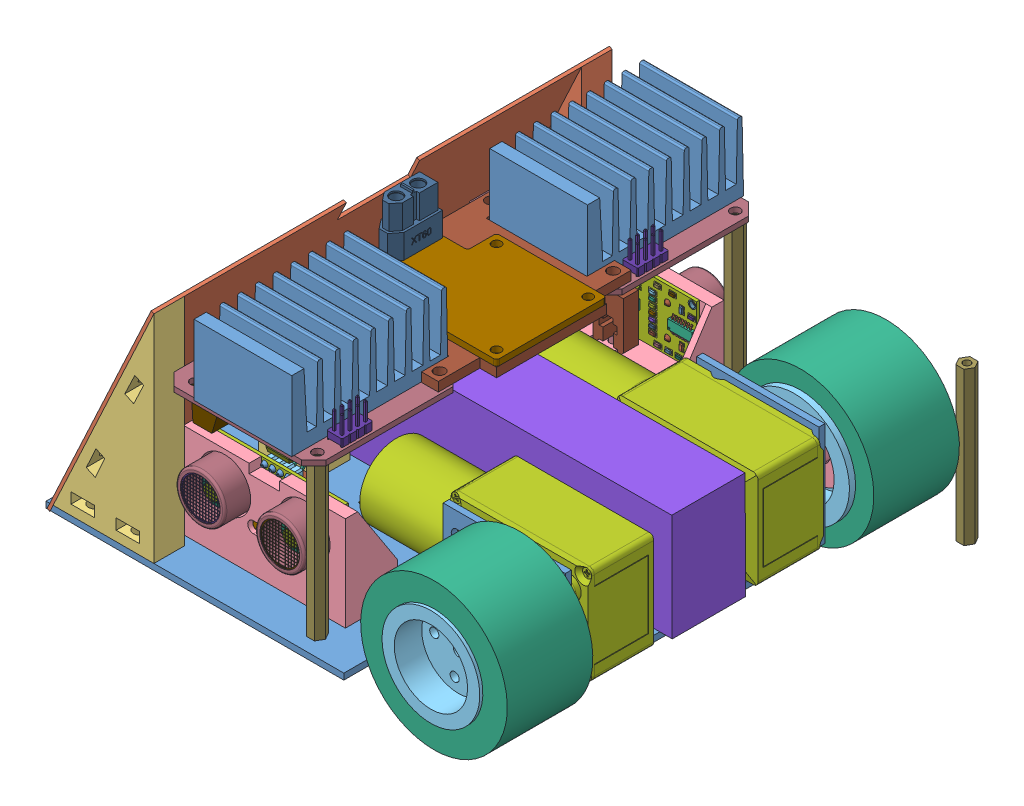
SolidWorks assembly sumover4, configuration Default. Lengths in mm.
Overall size (156.71 90.51 158.03).
240 component instances, 83 part files, 55 mates.
Components (placement in the parent):
- de_ver4-1: de_ver4 [Default] at (25.2124 85.45 125.8275) size (137.5 34 150)
- part_do_mui_phai-1: part_do_mui_phai [Default] at (-8.2076 87.45 60.8275) x (-1 0 0) z (0 0 -1) size (33 75.77 10)
- part_do_mui-1: part_do_mui [Default] at (-8.2076 87.45 200.8275) x (-1 0 0) z (0 0 -1) size (33 75.77 10)
- cum_mat_hai_ben-1: cum_mat_hai_ben [Default] at (15.9657 73.6076 21.8207) size (53 36.57 25)
  - ga lap ultrasonic v6-1: ga lap ultrasonic v6 [Default] at (-15.0838 26.1355 42.0068) size (53 31 17)
  - HC-04HC-04-1: HC-04HC-04 [Default] at (-1.0033 34.8424 47.0068) x (1 0 0) z (0 0 -1) size (45 25.57 17.46)
    - HC-04HC-04.stp-1: HC-04HC-04.stp [Default] at origin size (45 25.57 17.46)
      - HC-04Array.stp-1: HC-04Array.stp [Default] at origin size (10.16 2.54 2.54)
      - HC-04Array001.stp-1: HC-04Array001.stp [Default] at (0 0 1) size (8.32 7.52 6.46)
      - HC-04Placa.stp-1: HC-04Placa.stp [Default] at origin size (45 20 1)
      - HC-04Pad003.stp-1: HC-04Pad003.stp [Default] at (0 0 1) size (10.52 3.38 0.2)
      - HC-04Fillet.stp-1: HC-04Fillet.stp [Default] at (0 0 1) size (10.1 2.84 3)
      - HC-04Array002.stp-1: HC-04Array002.stp [Default] at origin size (9.62 2 1)
      - HC-04Array003.stp-1: HC-04Array003.stp [Default] at (0 0 1) size (28 12 0.8)
      - HC-04Fusion.stp-1: HC-04Fusion.stp [Default] at origin size (6 2 1)
      - HC-04Fillet001.stp-1: HC-04Fillet001.stp [Default] at (0 0 1) size (42 16 12)
      - HC-04Pad005.stp-1: HC-04Pad005.stp [Default] at (0 0 1) size (39.16 13 0.2)
      - HC-04Pad006.stp-1: HC-04Pad006.stp [Default] at (0 0 1) size (35.01 9.04 7)
      - HC-04Fusion001.stp-1: HC-04Fusion001.stp [Default] at (0 0 8) size (31 5 1.5)
      - HC-04Clone_of_Fusion002.stp-1: HC-04Clone_of_Fusion002.stp [Default] at (47.2 -5.5 12.6) size (13 13 0.15)
      - HC-04Clone_of_Fusion003.stp-1: HC-04Clone_of_Fusion003.stp [Default] at (21.2 -5.5 12.6) size (13 13 0.15)
      - HC-04Array005.stp-1: HC-04Array005.stp [Default] at origin size (9.62 2 1)
      - HC-04Array002002.stp-1: HC-04Array002002.stp [Default] at (-5.9 0.1 0.15) size (6.57 1.4 0.56)
      - HC-04Clone_of_Array002002.stp-1: HC-04Clone_of_Array002002.stp [Default] at (-23.9 0.1 0.15) size (6.57 1.4 0.56)
      - HC-04Array002003.stp-1: HC-04Array002003.stp [Default] at (-6.05 0 0.15) size (6.57 1.4 0.56)
      - HC-04Clone_of_Array002003.stp-1: HC-04Clone_of_Array002003.stp [Default] at (-24.05 0 0.15) size (6.57 1.4 0.56)
      - HC-04Integrados.stp-1: HC-04Integrados.stp [Default] at origin size (42.14 9 1)
      - HC-04ShapeString.stp-1: HC-04ShapeString.stp [Default] at (-3.2 -7 1.01) x (0 1 0) z (0 0 1) size (2.53 1.13 0.01)
      - HC-04ShapeString001.stp-1: HC-04ShapeString001.stp [Default] at (-0.6 -7 1.01) x (0 1 0) z (0 0 1) size (2.66 1.45 0.01)
      - HC-04ShapeString002.stp-1: HC-04ShapeString002.stp [Default] at (1.9 -7 1.01) x (0 1 0) z (0 0 1) size (3.21 1.16 0.01)
      - HC-04ShapeString003.stp-1: HC-04ShapeString003.stp [Default] at (4.5 -7 1.01) x (0 1 0) z (0 0 1) size (2.71 1.16 0.01)
      - HC-04ShapeString004.stp-1: HC-04ShapeString004.stp [Default] at (-19.5 -9.3 1.01) size (1.84 2.34 0.01)
      - HC-04ShapeString005.stp-1: HC-04ShapeString005.stp [Default] at (17.5 -9.3 1.01) size (1.82 2.34 0.01)
      - HC-04ShapeString006.stp-1: HC-04ShapeString006.stp [Default] at (-3 3.7 1.01) size (5.52 1.41 0.01)
      - HC-04Pad008.stp-1: HC-04Pad008.stp [Default] at (0 0 -0.01) size (44.56 19.6 1.02)
      - HC-04Scale004.stp-1: HC-04Scale004.stp [Default] at (-1.9 -21.5 -1.5) x (0 1 0) z (0 0 1) size (0.8 1.77 0.5)
      - HC-04Scale027.stp-1: HC-04Scale027.stp [Default] at (-1.9 -10.2323 -1.5) x (0 1 0) z (0 0 1) size (0.8 1.77 0.5)
      - HC-04Scale028.stp-1: HC-04Scale028.stp [Default] at (8.5984 -21.5 -1.5) x (0 1 0) z (0 0 1) size (0.8 1.77 0.5)
      - HC-04Scale029.stp-1: HC-04Scale029.stp [Default] at (8.5984 -19.5867 -1.5) x (0 1 0) z (0 0 1) size (0.8 1.77 0.5)
      - HC-04Scale030.stp-1: HC-04Scale030.stp [Default] at (8.5984 -17.5982 -1.5) x (0 1 0) z (0 0 1) size (0.8 1.77 0.5)
      - HC-04Scale031.stp-1: HC-04Scale031.stp [Default] at (8.5984 -15.6427 -1.5) x (0 1 0) z (0 0 1) size (0.8 1.77 0.5)
      - HC-04Scale032.stp-1: HC-04Scale032.stp [Default] at (8.5984 -11.6848 -1.5) x (0 1 0) z (0 0 1) size (0.8 1.77 0.5)
      - HC-04Scale033.stp-1: HC-04Scale033.stp [Default] at (-26.74 -2 -1.5) x (0 1 0) z (0 0 1) size (0.8 1.85 0.5)
      - HC-04Scale034.stp-1: HC-04Scale034.stp [Default] at (24.9371 -21.5 -1.5) x (0 1 0) z (0 0 1) size (0.8 1.77 0.5)
      - HC-04Scale035.stp-1: HC-04Scale035.stp [Default] at (24.9691 -19.5867 -1.5) x (0 1 0) z (0 0 1) size (0.8 1.77 0.5)
      - HC-04Scale036.stp-1: HC-04Scale036.stp [Default] at (24.9742 -17.5982 -1.5) x (0 1 0) z (0 0 1) size (0.8 1.77 0.5)
      - HC-04Scale037.stp-1: HC-04Scale037.stp [Default] at (-10.4013 -2 -1.5) x (0 1 0) z (0 0 1) size (0.8 1.85 0.5)
      - HC-04Scale038.stp-1: HC-04Scale038.stp [Default] at (-10.4013 -3.9266 -1.5) x (0 1 0) z (0 0 1) size (0.8 1.85 0.5)
      - HC-04Scale039.stp-1: HC-04Scale039.stp [Default] at (-10.4013 -0.0734 -1.5) x (0 1 0) z (0 0 1) size (0.8 1.85 0.5)
      - HC-04Scale040.stp-1: HC-04Scale040.stp [Default] at (24.9742 -9.855 -1.5) x (0 1 0) z (0 0 1) size (0.8 1.77 0.5)
      - HC-04Scale041.stp-1: HC-04Scale041.stp [Default] at (26.5673 -24.0564 -1.5) x (0 1 0) z (0 0 1) size (0.8 1.77 0.5)
      - HC-04Scale042.stp-1: HC-04Scale042.stp [Default] at (26.5673 -7.3333 -1.5) x (0 1 0) z (0 0 1) size (0.8 1.77 0.5)
      - HC-04Scale043.stp-1: HC-04Scale043.stp [Default] at (30.1435 -7.3333 -1.5) x (0 1 0) z (0 0 1) size (0.8 1.77 0.5)
      - HC-04Scale044.stp-1: HC-04Scale044.stp [Default] at (33.5459 -7.3333 -1.5) x (0 1 0) z (0 0 1) size (0.8 1.77 0.5)
      - HC-04Scale045.stp-1: HC-04Scale045.stp [Default] at (37.7181 -11.1827 -1.5) x (0 1 0) z (0 0 1) size (0.8 1.77 0.5)
      - HC-04Scale046.stp-1: HC-04Scale046.stp [Default] at (37.7181 -20.5932 -1.5) x (0 1 0) z (0 0 1) size (0.8 1.77 0.5)
      - HC-04Scale047.stp-1: HC-04Scale047.stp [Default] at (-3.9042 -12.3288 -1.5) x (0 1 0) z (0 0 1) size (0.8 1.85 0.5)
      - HC-04Scale048.stp-1: HC-04Scale048.stp [Default] at (13.5402 13.2894 -1.5) size (0.8 1.85 0.5)
      - HC-04Scale049.stp-1: HC-04Scale049.stp [Default] at (13.5402 23.7909 -1.5) size (0.8 1.85 0.5)
      - HC-04Pad009.stp-1: HC-04Pad009.stp [Default] x (1 0 0) z (0 0 -1) size (42.21 18.43 0.01)
      - HC-04ShapeString007.stp-1: HC-04ShapeString007.stp [Default] at (-3.2 -7 -0.1) x (0 1 0) z (0 0 1) size (2.53 1.13 0.01)
      - HC-04ShapeString008.stp-1: HC-04ShapeString008.stp [Default] at (-0.6 -7 -0.1) x (0 1 0) z (0 0 1) size (2.66 1.45 0.01)
      - HC-04ShapeString009.stp-1: HC-04ShapeString009.stp [Default] at (1.9 -7 -0.1) x (0 1 0) z (0 0 1) size (3.21 1.16 0.01)
      - HC-04ShapeString010.stp-1: HC-04ShapeString010.stp [Default] at (4.5 -7 -0.1) x (0 1 0) z (0 0 1) size (2.71 1.16 0.01)
      - HC-04Fusion002.stp-1: HC-04Fusion002.stp [Default] at origin size (5.7 7.57 0.56)
      - HC-04ShapeString011.stp-1: HC-04ShapeString011.stp [Default] at (-17.5 8.4 1.1) size (7.91 1.16 0.01)
      - HC-04ShapeString012.stp-1: HC-04ShapeString012.stp [Default] at (-7.5 8 -0.1) x (-1 0 0) z (0 0 -1) size (7.91 1.16 0.01)
  - 12.ganh-1: 12.ganh [Default] at (-1.0033 30.7424 48.5068) x (1 0 0) z (0 -1 0) size (10 5 19)
- cum_mat_hai_ben-2: cum_mat_hai_ben [Default] at (13.9591 73.6076 229.8343) x (-1 0 0) z (0 0 -1) size (53 36.57 25)
  - ga lap ultrasonic v6-1: ga lap ultrasonic v6 [Default] at (-15.0838 26.1355 42.0068) size (53 31 17)
  - HC-04HC-04-1: HC-04HC-04 [Default] at (-1.0033 34.8424 47.0068) x (1 0 0) z (0 0 -1) size (45 25.57 17.46)
    - HC-04HC-04.stp-1: HC-04HC-04.stp [Default] at origin size (45 25.57 17.46)
      - HC-04Array.stp-1: HC-04Array.stp [Default] at origin size (10.16 2.54 2.54)
      - HC-04Array001.stp-1: HC-04Array001.stp [Default] at (0 0 1) size (8.32 7.52 6.46)
      - HC-04Placa.stp-1: HC-04Placa.stp [Default] at origin size (45 20 1)
      - HC-04Pad003.stp-1: HC-04Pad003.stp [Default] at (0 0 1) size (10.52 3.38 0.2)
      - HC-04Fillet.stp-1: HC-04Fillet.stp [Default] at (0 0 1) size (10.1 2.84 3)
      - HC-04Array002.stp-1: HC-04Array002.stp [Default] at origin size (9.62 2 1)
      - HC-04Array003.stp-1: HC-04Array003.stp [Default] at (0 0 1) size (28 12 0.8)
      - HC-04Fusion.stp-1: HC-04Fusion.stp [Default] at origin size (6 2 1)
      - HC-04Fillet001.stp-1: HC-04Fillet001.stp [Default] at (0 0 1) size (42 16 12)
      - HC-04Pad005.stp-1: HC-04Pad005.stp [Default] at (0 0 1) size (39.16 13 0.2)
      - HC-04Pad006.stp-1: HC-04Pad006.stp [Default] at (0 0 1) size (35.01 9.04 7)
      - HC-04Fusion001.stp-1: HC-04Fusion001.stp [Default] at (0 0 8) size (31 5 1.5)
      - HC-04Clone_of_Fusion002.stp-1: HC-04Clone_of_Fusion002.stp [Default] at (47.2 -5.5 12.6) size (13 13 0.15)
      - HC-04Clone_of_Fusion003.stp-1: HC-04Clone_of_Fusion003.stp [Default] at (21.2 -5.5 12.6) size (13 13 0.15)
      - HC-04Array005.stp-1: HC-04Array005.stp [Default] at origin size (9.62 2 1)
      - HC-04Array002002.stp-1: HC-04Array002002.stp [Default] at (-5.9 0.1 0.15) size (6.57 1.4 0.56)
      - HC-04Clone_of_Array002002.stp-1: HC-04Clone_of_Array002002.stp [Default] at (-23.9 0.1 0.15) size (6.57 1.4 0.56)
      - HC-04Array002003.stp-1: HC-04Array002003.stp [Default] at (-6.05 0 0.15) size (6.57 1.4 0.56)
      - HC-04Clone_of_Array002003.stp-1: HC-04Clone_of_Array002003.stp [Default] at (-24.05 0 0.15) size (6.57 1.4 0.56)
      - HC-04Integrados.stp-1: HC-04Integrados.stp [Default] at origin size (42.14 9 1)
      - HC-04ShapeString.stp-1: HC-04ShapeString.stp [Default] at (-3.2 -7 1.01) x (0 1 0) z (0 0 1) size (2.53 1.13 0.01)
      - HC-04ShapeString001.stp-1: HC-04ShapeString001.stp [Default] at (-0.6 -7 1.01) x (0 1 0) z (0 0 1) size (2.66 1.45 0.01)
      - HC-04ShapeString002.stp-1: HC-04ShapeString002.stp [Default] at (1.9 -7 1.01) x (0 1 0) z (0 0 1) size (3.21 1.16 0.01)
      - HC-04ShapeString003.stp-1: HC-04ShapeString003.stp [Default] at (4.5 -7 1.01) x (0 1 0) z (0 0 1) size (2.71 1.16 0.01)
      - HC-04ShapeString004.stp-1: HC-04ShapeString004.stp [Default] at (-19.5 -9.3 1.01) size (1.84 2.34 0.01)
      - HC-04ShapeString005.stp-1: HC-04ShapeString005.stp [Default] at (17.5 -9.3 1.01) size (1.82 2.34 0.01)
      - HC-04ShapeString006.stp-1: HC-04ShapeString006.stp [Default] at (-3 3.7 1.01) size (5.52 1.41 0.01)
      - HC-04Pad008.stp-1: HC-04Pad008.stp [Default] at (0 0 -0.01) size (44.56 19.6 1.02)
      - HC-04Scale004.stp-1: HC-04Scale004.stp [Default] at (-1.9 -21.5 -1.5) x (0 1 0) z (0 0 1) size (0.8 1.77 0.5)
      - HC-04Scale027.stp-1: HC-04Scale027.stp [Default] at (-1.9 -10.2323 -1.5) x (0 1 0) z (0 0 1) size (0.8 1.77 0.5)
      - HC-04Scale028.stp-1: HC-04Scale028.stp [Default] at (8.5984 -21.5 -1.5) x (0 1 0) z (0 0 1) size (0.8 1.77 0.5)
      - HC-04Scale029.stp-1: HC-04Scale029.stp [Default] at (8.5984 -19.5867 -1.5) x (0 1 0) z (0 0 1) size (0.8 1.77 0.5)
      - HC-04Scale030.stp-1: HC-04Scale030.stp [Default] at (8.5984 -17.5982 -1.5) x (0 1 0) z (0 0 1) size (0.8 1.77 0.5)
      - HC-04Scale031.stp-1: HC-04Scale031.stp [Default] at (8.5984 -15.6427 -1.5) x (0 1 0) z (0 0 1) size (0.8 1.77 0.5)
      - HC-04Scale032.stp-1: HC-04Scale032.stp [Default] at (8.5984 -11.6848 -1.5) x (0 1 0) z (0 0 1) size (0.8 1.77 0.5)
      - HC-04Scale033.stp-1: HC-04Scale033.stp [Default] at (-26.74 -2 -1.5) x (0 1 0) z (0 0 1) size (0.8 1.85 0.5)
      - HC-04Scale034.stp-1: HC-04Scale034.stp [Default] at (24.9371 -21.5 -1.5) x (0 1 0) z (0 0 1) size (0.8 1.77 0.5)
      - HC-04Scale035.stp-1: HC-04Scale035.stp [Default] at (24.9691 -19.5867 -1.5) x (0 1 0) z (0 0 1) size (0.8 1.77 0.5)
      - HC-04Scale036.stp-1: HC-04Scale036.stp [Default] at (24.9742 -17.5982 -1.5) x (0 1 0) z (0 0 1) size (0.8 1.77 0.5)
      - HC-04Scale037.stp-1: HC-04Scale037.stp [Default] at (-10.4013 -2 -1.5) x (0 1 0) z (0 0 1) size (0.8 1.85 0.5)
      - HC-04Scale038.stp-1: HC-04Scale038.stp [Default] at (-10.4013 -3.9266 -1.5) x (0 1 0) z (0 0 1) size (0.8 1.85 0.5)
      - HC-04Scale039.stp-1: HC-04Scale039.stp [Default] at (-10.4013 -0.0734 -1.5) x (0 1 0) z (0 0 1) size (0.8 1.85 0.5)
      - HC-04Scale040.stp-1: HC-04Scale040.stp [Default] at (24.9742 -9.855 -1.5) x (0 1 0) z (0 0 1) size (0.8 1.77 0.5)
      - HC-04Scale041.stp-1: HC-04Scale041.stp [Default] at (26.5673 -24.0564 -1.5) x (0 1 0) z (0 0 1) size (0.8 1.77 0.5)
      - HC-04Scale042.stp-1: HC-04Scale042.stp [Default] at (26.5673 -7.3333 -1.5) x (0 1 0) z (0 0 1) size (0.8 1.77 0.5)
      - HC-04Scale043.stp-1: HC-04Scale043.stp [Default] at (30.1435 -7.3333 -1.5) x (0 1 0) z (0 0 1) size (0.8 1.77 0.5)
      - HC-04Scale044.stp-1: HC-04Scale044.stp [Default] at (33.5459 -7.3333 -1.5) x (0 1 0) z (0 0 1) size (0.8 1.77 0.5)
      - HC-04Scale045.stp-1: HC-04Scale045.stp [Default] at (37.7181 -11.1827 -1.5) x (0 1 0) z (0 0 1) size (0.8 1.77 0.5)
      - HC-04Scale046.stp-1: HC-04Scale046.stp [Default] at (37.7181 -20.5932 -1.5) x (0 1 0) z (0 0 1) size (0.8 1.77 0.5)
      - HC-04Scale047.stp-1: HC-04Scale047.stp [Default] at (-3.9042 -12.3288 -1.5) x (0 1 0) z (0 0 1) size (0.8 1.85 0.5)
      - HC-04Scale048.stp-1: HC-04Scale048.stp [Default] at (13.5402 13.2894 -1.5) size (0.8 1.85 0.5)
      - HC-04Scale049.stp-1: HC-04Scale049.stp [Default] at (13.5402 23.7909 -1.5) size (0.8 1.85 0.5)
      - HC-04Pad009.stp-1: HC-04Pad009.stp [Default] x (1 0 0) z (0 0 -1) size (42.21 18.43 0.01)
      - HC-04ShapeString007.stp-1: HC-04ShapeString007.stp [Default] at (-3.2 -7 -0.1) x (0 1 0) z (0 0 1) size (2.53 1.13 0.01)
      - HC-04ShapeString008.stp-1: HC-04ShapeString008.stp [Default] at (-0.6 -7 -0.1) x (0 1 0) z (0 0 1) size (2.66 1.45 0.01)
      - HC-04ShapeString009.stp-1: HC-04ShapeString009.stp [Default] at (1.9 -7 -0.1) x (0 1 0) z (0 0 1) size (3.21 1.16 0.01)
      - HC-04ShapeString010.stp-1: HC-04ShapeString010.stp [Default] at (4.5 -7 -0.1) x (0 1 0) z (0 0 1) size (2.71 1.16 0.01)
      - HC-04Fusion002.stp-1: HC-04Fusion002.stp [Default] at origin size (5.7 7.57 0.56)
      - HC-04ShapeString011.stp-1: HC-04ShapeString011.stp [Default] at (-17.5 8.4 1.1) size (7.91 1.16 0.01)
      - HC-04ShapeString012.stp-1: HC-04ShapeString012.stp [Default] at (-7.5 8 -0.1) x (-1 0 0) z (0 0 -1) size (7.91 1.16 0.01)
  - 12.ganh-1: 12.ganh [Default] at (-1.0033 30.7424 48.5068) x (1 0 0) z (0 -1 0) size (10 5 19)
- truc_dong_50mm-1: truc_dong_50mm [Default] at (38.7124 87.45 194.2275) size (5.31 50 4.6)
- truc_dong_50mm-2: truc_dong_50mm [Default] at (-1.2876 87.45 154.2275) x (-0.99996 0 -0.00896) z (0.00896 0 -0.99996) size (5.31 50 4.6)
- truc_dong_50mm-3: truc_dong_50mm [Default] at (-1.2876 87.45 97.4275) x (-0.99996 0 -0.00896) z (0.00896 0 -0.99996) size (5.31 50 4.6)
- truc_dong_50mm-4: truc_dong_50mm [Default] at (38.7124 87.45 57.4275) x (-0.99996 0 -0.00896) z (0.00896 0 -0.99996) size (5.31 50 4.6)
- BTS_co_tan_nhiet-1: BTS_co_tan_nhiet [Default] at (-58.0066 153.9561 222.7544) x (0 0 1) z (1 0 0) size (51 42.4 49.96)
  - 8.BTS7960 43A HIGH POWER H BRIDGE MODULE-1: 8.BTS7960 43A HIGH POWER H BRIDGE MODULE [Default] at (-48.5269 14.8061 75.419) size (49.5 27.9 49.96)
    - PCB, BTS7960 43A HIGH POWER H BRIDGE MODULE-1: PCB, BTS7960 43A HIGH POWER H BRIDGE MODULE [Default] at origin size (49.5 1.7 49.8)
    - ALUMINUM ELECTROLYTIC CAPACITOR, 330 uF, BTS7960 43A HIGH POWER H BRIDGE MODULE-1: ALUMINUM ELECTROLYTIC CAPACITOR, 330 uF, BTS7960 43A HIGH POWER H BRIDGE MODULE [Default] at (-10.75 1.8 -19.85) x (0.999469 0 -0.032584) z (0.032584 0 0.999469) size (10.1 18.7 10.1)
    - BTN7960 IC, BTS7960 43A HIGH POWER H BRIDGE MODULE-1: BTN7960 IC, BTS7960 43A HIGH POWER H BRIDGE MODULE [Default] at (5.95 1.7 1.8) x (-1 0 0) z (0 0 -1) size (9.6 4.6 14.9)
    - BTN7960 IC, BTS7960 43A HIGH POWER H BRIDGE MODULE-2: BTN7960 IC, BTS7960 43A HIGH POWER H BRIDGE MODULE [Default] at (-5.95 1.7 1.8) x (-1 0 0) z (0 0 -1) size (9.6 4.6 14.9)
    - NXP 74HC244D, BUFFER AND LINE DRIVER, BTS7960 43A HIGH POWER H BRIDGE MODULE-1: NXP 74HC244D, BUFFER AND LINE DRIVER, BTS7960 43A HIGH POWER H BRIDGE MODULE [Default] at (17.35 3 12.1) size (13 2.6 10.4)
    - y 8 PIN HEADER, IC, BTS7960 43A HIGH POWER H BRIDGE MODULE-1: y 8 PIN HEADER, IC, BTS7960 43A HIGH POWER H BRIDGE MODULE [Default] at (-34.78 -2.5 22.83) x (0 0 1) z (-1 0 0) size (5.08 11.6 10.16)
    - EUROSTYLE TERMINAL BLOCK 2 POS 5.0 MM RA PLUG, BTS7960 43A HIGH POWER H BRIDGE MODULE-1: EUROSTYLE TERMINAL BLOCK 2 POS 5.0 MM RA PLUG, BTS7960 43A HIGH POWER H BRIDGE MODULE [Default] at (0.75 4.2 -6.5) size (10 14.5 10.5)
    - EUROSTYLE TERMINAL BLOCK 2 POS 5.0 MM RA PLUG, BTS7960 43A HIGH POWER H BRIDGE MODULE-2: EUROSTYLE TERMINAL BLOCK 2 POS 5.0 MM RA PLUG, BTS7960 43A HIGH POWER H BRIDGE MODULE [Default] at (10.75 4.2 -6.5) size (10 14.5 10.5)
  - HEATSINK, BTS7960 43A HIGH POWER H BRIDGE MODULE-1: HEATSINK, BTS7960 43A HIGH POWER H BRIDGE MODULE [Default] at (-48.5269 14.8061 77.819) size (51 23 32.02)
- BTS_co_tan_nhiet-2: BTS_co_tan_nhiet [Default] at (-58.0066 153.9561 125.9544) x (0 0 1) z (1 0 0) size (51 42.4 49.96)
  - 8.BTS7960 43A HIGH POWER H BRIDGE MODULE-1: 8.BTS7960 43A HIGH POWER H BRIDGE MODULE [Default] at (-48.5269 14.8061 75.419) size (49.5 27.9 49.96)
    - PCB, BTS7960 43A HIGH POWER H BRIDGE MODULE-1: PCB, BTS7960 43A HIGH POWER H BRIDGE MODULE [Default] at origin size (49.5 1.7 49.8)
    - ALUMINUM ELECTROLYTIC CAPACITOR, 330 uF, BTS7960 43A HIGH POWER H BRIDGE MODULE-1: ALUMINUM ELECTROLYTIC CAPACITOR, 330 uF, BTS7960 43A HIGH POWER H BRIDGE MODULE [Default] at (-10.75 1.8 -19.85) x (0.999469 0 -0.032584) z (0.032584 0 0.999469) size (10.1 18.7 10.1)
    - BTN7960 IC, BTS7960 43A HIGH POWER H BRIDGE MODULE-1: BTN7960 IC, BTS7960 43A HIGH POWER H BRIDGE MODULE [Default] at (5.95 1.7 1.8) x (-1 0 0) z (0 0 -1) size (9.6 4.6 14.9)
    - BTN7960 IC, BTS7960 43A HIGH POWER H BRIDGE MODULE-2: BTN7960 IC, BTS7960 43A HIGH POWER H BRIDGE MODULE [Default] at (-5.95 1.7 1.8) x (-1 0 0) z (0 0 -1) size (9.6 4.6 14.9)
    - NXP 74HC244D, BUFFER AND LINE DRIVER, BTS7960 43A HIGH POWER H BRIDGE MODULE-1: NXP 74HC244D, BUFFER AND LINE DRIVER, BTS7960 43A HIGH POWER H BRIDGE MODULE [Default] at (17.35 3 12.1) size (13 2.6 10.4)
    - y 8 PIN HEADER, IC, BTS7960 43A HIGH POWER H BRIDGE MODULE-1: y 8 PIN HEADER, IC, BTS7960 43A HIGH POWER H BRIDGE MODULE [Default] at (-34.78 -2.5 22.83) x (0 0 1) z (-1 0 0) size (5.08 11.6 10.16)
    - EUROSTYLE TERMINAL BLOCK 2 POS 5.0 MM RA PLUG, BTS7960 43A HIGH POWER H BRIDGE MODULE-1: EUROSTYLE TERMINAL BLOCK 2 POS 5.0 MM RA PLUG, BTS7960 43A HIGH POWER H BRIDGE MODULE [Default] at (0.75 4.2 -6.5) size (10 14.5 10.5)
    - EUROSTYLE TERMINAL BLOCK 2 POS 5.0 MM RA PLUG, BTS7960 43A HIGH POWER H BRIDGE MODULE-2: EUROSTYLE TERMINAL BLOCK 2 POS 5.0 MM RA PLUG, BTS7960 43A HIGH POWER H BRIDGE MODULE [Default] at (10.75 4.2 -6.5) size (10 14.5 10.5)
  - HEATSINK, BTS7960 43A HIGH POWER H BRIDGE MODULE-1: HEATSINK, BTS7960 43A HIGH POWER H BRIDGE MODULE [Default] at (-48.5269 14.8061 77.819) size (51 23 32.02)
- part_chan-1: part_chan [Default] at (-26.7813 120.7534 125.8275) x (0 0 -1) z (0.906308 -0.422618 0) size (150 80.6 1)
- ga lap ultrasonic v5-1: ga lap ultrasonic v5 [Default] at (-22.5376 103.7431 139.908) x (0 0 -1) z (1 0 0) size (53 35 17)
- HC-04HC-04-1: HC-04HC-04 [Default] at (-17.5376 112.45 125.8275) x (0 0 -1) z (-1 0 0) size (45 25.57 17.46)
  - HC-04HC-04.stp-1: HC-04HC-04.stp [Default] at origin size (45 25.57 17.46)
    - HC-04Array.stp-1: HC-04Array.stp [Default] at origin size (10.16 2.54 2.54)
    - HC-04Array001.stp-1: HC-04Array001.stp [Default] at (0 0 1) size (8.32 7.52 6.46)
    - HC-04Placa.stp-1: HC-04Placa.stp [Default] at origin size (45 20 1)
    - HC-04Pad003.stp-1: HC-04Pad003.stp [Default] at (0 0 1) size (10.52 3.38 0.2)
    - HC-04Fillet.stp-1: HC-04Fillet.stp [Default] at (0 0 1) size (10.1 2.84 3)
    - HC-04Array002.stp-1: HC-04Array002.stp [Default] at origin size (9.62 2 1)
    - HC-04Array003.stp-1: HC-04Array003.stp [Default] at (0 0 1) size (28 12 0.8)
    - HC-04Fusion.stp-1: HC-04Fusion.stp [Default] at origin size (6 2 1)
    - HC-04Fillet001.stp-1: HC-04Fillet001.stp [Default] at (0 0 1) size (42 16 12)
    - HC-04Pad005.stp-1: HC-04Pad005.stp [Default] at (0 0 1) size (39.16 13 0.2)
    - HC-04Pad006.stp-1: HC-04Pad006.stp [Default] at (0 0 1) size (35.01 9.04 7)
    - HC-04Fusion001.stp-1: HC-04Fusion001.stp [Default] at (0 0 8) size (31 5 1.5)
    - HC-04Clone_of_Fusion002.stp-1: HC-04Clone_of_Fusion002.stp [Default] at (47.2 -5.5 12.6) size (13 13 0.15)
    - HC-04Clone_of_Fusion003.stp-1: HC-04Clone_of_Fusion003.stp [Default] at (21.2 -5.5 12.6) size (13 13 0.15)
    - HC-04Array005.stp-1: HC-04Array005.stp [Default] at origin size (9.62 2 1)
    - HC-04Array002002.stp-1: HC-04Array002002.stp [Default] at (-5.9 0.1 0.15) size (6.57 1.4 0.56)
    - HC-04Clone_of_Array002002.stp-1: HC-04Clone_of_Array002002.stp [Default] at (-23.9 0.1 0.15) size (6.57 1.4 0.56)
    - HC-04Array002003.stp-1: HC-04Array002003.stp [Default] at (-6.05 0 0.15) size (6.57 1.4 0.56)
    - HC-04Clone_of_Array002003.stp-1: HC-04Clone_of_Array002003.stp [Default] at (-24.05 0 0.15) size (6.57 1.4 0.56)
    - HC-04Integrados.stp-1: HC-04Integrados.stp [Default] at origin size (42.14 9 1)
    - HC-04ShapeString.stp-1: HC-04ShapeString.stp [Default] at (-3.2 -7 1.01) x (0 1 0) z (0 0 1) size (2.53 1.13 0.01)
    - HC-04ShapeString001.stp-1: HC-04ShapeString001.stp [Default] at (-0.6 -7 1.01) x (0 1 0) z (0 0 1) size (2.66 1.45 0.01)
    - HC-04ShapeString002.stp-1: HC-04ShapeString002.stp [Default] at (1.9 -7 1.01) x (0 1 0) z (0 0 1) size (3.21 1.16 0.01)
    - HC-04ShapeString003.stp-1: HC-04ShapeString003.stp [Default] at (4.5 -7 1.01) x (0 1 0) z (0 0 1) size (2.71 1.16 0.01)
    - HC-04ShapeString004.stp-1: HC-04ShapeString004.stp [Default] at (-19.5 -9.3 1.01) size (1.84 2.34 0.01)
    - HC-04ShapeString005.stp-1: HC-04ShapeString005.stp [Default] at (17.5 -9.3 1.01) size (1.82 2.34 0.01)
    - HC-04ShapeString006.stp-1: HC-04ShapeString006.stp [Default] at (-3 3.7 1.01) size (5.52 1.41 0.01)
    - HC-04Pad008.stp-1: HC-04Pad008.stp [Default] at (0 0 -0.01) size (44.56 19.6 1.02)
    - HC-04Scale004.stp-1: HC-04Scale004.stp [Default] at (-1.9 -21.5 -1.5) x (0 1 0) z (0 0 1) size (0.8 1.77 0.5)
    - HC-04Scale027.stp-1: HC-04Scale027.stp [Default] at (-1.9 -10.2323 -1.5) x (0 1 0) z (0 0 1) size (0.8 1.77 0.5)
    - HC-04Scale028.stp-1: HC-04Scale028.stp [Default] at (8.5984 -21.5 -1.5) x (0 1 0) z (0 0 1) size (0.8 1.77 0.5)
    - HC-04Scale029.stp-1: HC-04Scale029.stp [Default] at (8.5984 -19.5867 -1.5) x (0 1 0) z (0 0 1) size (0.8 1.77 0.5)
    - HC-04Scale030.stp-1: HC-04Scale030.stp [Default] at (8.5984 -17.5982 -1.5) x (0 1 0) z (0 0 1) size (0.8 1.77 0.5)
    - HC-04Scale031.stp-1: HC-04Scale031.stp [Default] at (8.5984 -15.6427 -1.5) x (0 1 0) z (0 0 1) size (0.8 1.77 0.5)
    - HC-04Scale032.stp-1: HC-04Scale032.stp [Default] at (8.5984 -11.6848 -1.5) x (0 1 0) z (0 0 1) size (0.8 1.77 0.5)
    - HC-04Scale033.stp-1: HC-04Scale033.stp [Default] at (-26.74 -2 -1.5) x (0 1 0) z (0 0 1) size (0.8 1.85 0.5)
    - HC-04Scale034.stp-1: HC-04Scale034.stp [Default] at (24.9371 -21.5 -1.5) x (0 1 0) z (0 0 1) size (0.8 1.77 0.5)
    - HC-04Scale035.stp-1: HC-04Scale035.stp [Default] at (24.9691 -19.5867 -1.5) x (0 1 0) z (0 0 1) size (0.8 1.77 0.5)
    - HC-04Scale036.stp-1: HC-04Scale036.stp [Default] at (24.9742 -17.5982 -1.5) x (0 1 0) z (0 0 1) size (0.8 1.77 0.5)
    - HC-04Scale037.stp-1: HC-04Scale037.stp [Default] at (-10.4013 -2 -1.5) x (0 1 0) z (0 0 1) size (0.8 1.85 0.5)
    - HC-04Scale038.stp-1: HC-04Scale038.stp [Default] at (-10.4013 -3.9266 -1.5) x (0 1 0) z (0 0 1) size (0.8 1.85 0.5)
    - HC-04Scale039.stp-1: HC-04Scale039.stp [Default] at (-10.4013 -0.0734 -1.5) x (0 1 0) z (0 0 1) size (0.8 1.85 0.5)
    - HC-04Scale040.stp-1: HC-04Scale040.stp [Default] at (24.9742 -9.855 -1.5) x (0 1 0) z (0 0 1) size (0.8 1.77 0.5)
    - HC-04Scale041.stp-1: HC-04Scale041.stp [Default] at (26.5673 -24.0564 -1.5) x (0 1 0) z (0 0 1) size (0.8 1.77 0.5)
    - HC-04Scale042.stp-1: HC-04Scale042.stp [Default] at (26.5673 -7.3333 -1.5) x (0 1 0) z (0 0 1) size (0.8 1.77 0.5)
    - HC-04Scale043.stp-1: HC-04Scale043.stp [Default] at (30.1435 -7.3333 -1.5) x (0 1 0) z (0 0 1) size (0.8 1.77 0.5)
    - HC-04Scale044.stp-1: HC-04Scale044.stp [Default] at (33.5459 -7.3333 -1.5) x (0 1 0) z (0 0 1) size (0.8 1.77 0.5)
    - HC-04Scale045.stp-1: HC-04Scale045.stp [Default] at (37.7181 -11.1827 -1.5) x (0 1 0) z (0 0 1) size (0.8 1.77 0.5)
    - HC-04Scale046.stp-1: HC-04Scale046.stp [Default] at (37.7181 -20.5932 -1.5) x (0 1 0) z (0 0 1) size (0.8 1.77 0.5)
    - HC-04Scale047.stp-1: HC-04Scale047.stp [Default] at (-3.9042 -12.3288 -1.5) x (0 1 0) z (0 0 1) size (0.8 1.85 0.5)
    - HC-04Scale048.stp-1: HC-04Scale048.stp [Default] at (13.5402 13.2894 -1.5) size (0.8 1.85 0.5)
    - HC-04Scale049.stp-1: HC-04Scale049.stp [Default] at (13.5402 23.7909 -1.5) size (0.8 1.85 0.5)
    - HC-04Pad009.stp-1: HC-04Pad009.stp [Default] x (1 0 0) z (0 0 -1) size (42.21 18.43 0.01)
    - HC-04ShapeString007.stp-1: HC-04ShapeString007.stp [Default] at (-3.2 -7 -0.1) x (0 1 0) z (0 0 1) size (2.53 1.13 0.01)
    - HC-04ShapeString008.stp-1: HC-04ShapeString008.stp [Default] at (-0.6 -7 -0.1) x (0 1 0) z (0 0 1) size (2.66 1.45 0.01)
    - HC-04ShapeString009.stp-1: HC-04ShapeString009.stp [Default] at (1.9 -7 -0.1) x (0 1 0) z (0 0 1) size (3.21 1.16 0.01)
    - HC-04ShapeString010.stp-1: HC-04ShapeString010.stp [Default] at (4.5 -7 -0.1) x (0 1 0) z (0 0 1) size (2.71 1.16 0.01)
    - HC-04Fusion002.stp-1: HC-04Fusion002.stp [Default] at origin size (5.7 7.57 0.56)
    - HC-04ShapeString011.stp-1: HC-04ShapeString011.stp [Default] at (-17.5 8.4 1.1) size (7.91 1.16 0.01)
    - HC-04ShapeString012.stp-1: HC-04ShapeString012.stp [Default] at (-7.5 8 -0.1) x (-1 0 0) z (0 0 -1) size (7.91 1.16 0.01)
- 12.ganh-1: 12.ganh [Default] at (-11.0376 108.35 125.8275) x (0 0 1) z (0 -1 0) size (10 5 19)
- banhxe-1: banhxe [Default] at (52.3102 164.6143 71.5756) x (0.338518 0.94096 0) z (0.94096 -0.338518 0) size (48 34 48)
  - mat_bich_phi6-1: mat_bich_phi6 [Default] at (-47.3462 1.2519 49.0772) size (22 12 22)
  - 13.LoiBanhVer3-1: 13.LoiBanhVer3 [Default] at (-47.3462 -5.7481 49.0772) x (0 -1 0) z (0 0 1) size (31 36 36)
  - 2.lop_banh_xe-1: 2.lop_banh_xe [Default] at (-47.3462 -19.7481 49.0772) x (1 0 0) z (0 1 0) size (48 48 28)
- 4.JGY370_Reduction DC Motor-6mm-2: 4.JGY370_Reduction DC Motor-6mm [Default] at (82.4624 103.45 162.3275) x (-1 0 0) z (0 1 0) size (80.2 40.2 32)
- banhxe-3: banhxe [Default] at (121.8297 47.7682 180.0794) x (0.988465 -0.151451 0) z (0.151451 0.988465 0) size (48 34 48)
  - mat_bich_phi6-1: mat_bich_phi6 [Default] at (-47.3462 1.2519 49.0772) size (22 12 22)
  - 13.LoiBanhVer3-1: 13.LoiBanhVer3 [Default] at (-47.3462 -5.7481 49.0772) x (0 -1 0) z (0 0 1) size (31 36 36)
  - 2.lop_banh_xe-1: 2.lop_banh_xe [Default] at (-47.3462 -19.7481 49.0772) x (1 0 0) z (0 1 0) size (48 48 28)
- 4.JGY370_Reduction DC Motor-6mm-3: 4.JGY370_Reduction DC Motor-6mm [Default] at (82.4624 103.45 89.3275) x (-1 0 0) z (0 -1 0) size (80.2 40.2 32)
- 9.pin-1: 9.pin [Default] at (98.3893 105.3868 125.8275) x (0.004123 -0.999992 0) z (-0.999992 -0.004123 0) size (35 24 106)
- Machchianguon-1: Machchianguon [Default] at (35.7033 112.7735 164.9544) x (-1 0 0) z (0 0 -1) size (51 21.15 36)
  - mach_chia_nguon-1: mach_chia_nguon [Default] at (-11.2591 29.3765 57.1219) size (51 2 36)
  - Component1.step-1: Component1.step [Default] at (39.7409 31.3765 46.9219) x (0 0 -1) z (0 1 0) size (15.6 7.5 21.15)
- part_do_mach_chia_nguon-1: part_do_mach_chia_nguon [Default] at (18.7124 139.15 125.8325) x (-1 0 0) z (0 1 0) size (51 63.15 3)
- truc_dong_50mm-5: truc_dong_50mm [Default] at (102.1964 71.6421 45.0966) size (5.31 50 4.6)
Mates (geometry in assembly coordinates):
- Coincident1: coincident anti-aligned: plane of de_ver4-1 through (25.2124 87.45 125.8275) normal (0 1 0); plane of part_do_mui_phai-1 through (-8.2076 87.45 50.8275) normal (0 -1 0)
- Width1: width anti-aligned: plane of part_do_mui_phai-1 through (-21.7076 82.45 53.8275) normal (0 0 -1); plane of de_ver4-1 through (-21.7076 82.45 57.8275) normal (0 0 1); plane of part_do_mui_phai-1 through (-21.7076 87.45 53.8275) normal (0 0 1); plane of de_ver4-1 through (-27.7076 87.45 57.8275) normal (0 0 -1)
- Width2: width anti-aligned: plane of part_do_mui_phai-1 through (-21.7076 82.45 53.8275) normal (1 0 0); plane of de_ver4-1 through (-27.7076 82.45 53.8275) normal (-1 0 0); plane of part_do_mui_phai-1 through (-21.7076 87.45 57.8275) normal (-1 0 0); plane of de_ver4-1 through (-27.7076 87.45 53.8275) normal (1 0 0)
- Coincident2: coincident anti-aligned: plane of de_ver4-1 through (25.2124 87.45 125.8275) normal (0 1 0); plane of part_do_mui-1 through (-8.2076 87.45 190.8275) normal (0 -1 0)
- Width3: width aligned: plane of part_do_mui-1 through (-21.7076 82.45 197.8275) normal (0 0 1); plane of de_ver4-1 through (-21.7076 82.45 193.8275) normal (0 0 -1); plane of part_do_mui-1 through (-27.7076 87.45 193.8275) normal (0 0 1); plane of de_ver4-1 through (-21.7076 87.45 197.8275) normal (0 0 -1)
- Width4: width anti-aligned: plane of de_ver4-1 through (-27.7076 87.45 197.8275) normal (1 0 0); plane of part_do_mui-1 through (-21.7076 87.45 193.8275) normal (-1 0 0); plane of de_ver4-1 through (-27.7076 82.45 193.8275) normal (-1 0 0); plane of part_do_mui-1 through (-21.7076 82.45 193.8275) normal (1 0 0)
- Coincident3: coincident anti-aligned: plane of de_ver4-1 through (25.2124 87.45 125.8275) normal (0 1 0); plane of cum_mat_hai_ben-1/ga lap ultrasonic v6-1 through (0.8819 87.45 63.8275) normal (0 -1 0)
- Concentric1: concentric anti-aligned: cylinder of de_ver4-1 through (-4.5376 87.45 75.8275) axis (0 -1 0) radius 1.75; cylinder of cum_mat_hai_ben-1/ga lap ultrasonic v6-1 through (-4.5376 93.45 75.8275) axis (0 1 0) radius 1.75
- Concentric2: concentric anti-aligned: cylinder of de_ver4-1 through (34.4624 87.45 75.8275) axis (0 -1 0) radius 1.75; cylinder of cum_mat_hai_ben-1/ga lap ultrasonic v6-1 through (34.4624 93.45 75.8275) axis (0 1 0) radius 1.75
- Coincident4: coincident anti-aligned: plane of de_ver4-1 through (25.2124 87.45 125.8275) normal (0 1 0); plane of cum_mat_hai_ben-2/ga lap ultrasonic v6-1 through (29.0429 87.45 187.8275) normal (0 -1 0)
- Concentric3: concentric anti-aligned: cylinder of de_ver4-1 through (34.4624 87.45 175.8275) axis (0 -1 0) radius 1.75; cylinder of cum_mat_hai_ben-2/ga lap ultrasonic v6-1 through (34.4624 93.45 175.8275) axis (0 1 0) radius 1.75
- Concentric4: concentric anti-aligned: cylinder of de_ver4-1 through (-4.5376 87.45 175.8275) axis (0 -1 0) radius 1.75; cylinder of cum_mat_hai_ben-2/ga lap ultrasonic v6-1 through (-4.5376 93.45 175.8275) axis (0 1 0) radius 1.75
- Coincident5: coincident anti-aligned: plane of de_ver4-1 through (25.2124 87.45 125.8275) normal (0 1 0); plane of truc_dong_50mm-1 through (38.7124 87.45 194.2275) normal (0 -1 0)
- Concentric5: concentric aligned: cylinder of de_ver4-1 through (38.7124 87.45 194.2275) axis (0 -1 0) radius 1.75; cylinder of truc_dong_50mm-1 through (38.7124 137.45 194.2275) axis (0 -1 0) radius 1.2
- Concentric6: concentric aligned: cylinder of de_ver4-1 through (-1.2876 87.45 154.2275) axis (0 -1 0) radius 1.75; cylinder of truc_dong_50mm-2 through (-1.2876 137.45 154.2275) axis (0 -1 0) radius 1.2
- Coincident6: coincident anti-aligned: plane of de_ver4-1 through (25.2124 87.45 125.8275) normal (0 1 0); plane of truc_dong_50mm-2 through (-1.2876 87.45 154.2275) normal (0 -1 0)
- Coincident7: coincident anti-aligned: plane of de_ver4-1 through (25.2124 87.45 125.8275) normal (0 1 0); plane of truc_dong_50mm-3 through (-1.2876 87.45 97.4275) normal (0 -1 0)
- Coincident8: coincident anti-aligned: plane of de_ver4-1 through (25.2124 87.45 125.8275) normal (0 1 0); plane of truc_dong_50mm-4 through (38.7124 87.45 57.4275) normal (0 -1 0)
- Concentric7: concentric aligned: cylinder of de_ver4-1 through (38.7124 87.45 57.4275) axis (0 -1 0) radius 1.75; cylinder of truc_dong_50mm-4 through (38.7124 137.45 57.4275) axis (0 -1 0) radius 1.2
- Coincident9: coincident anti-aligned: plane of truc_dong_50mm-1 through (38.7124 137.45 194.2275) normal (0 1 0); plane of BTS_co_tan_nhiet-1/8.BTS7960 43A HIGH POWER H BRIDGE MODULE-1/PCB, BTS7960 43A HIGH POWER H BRIDGE MODULE-1 through (17.4124 137.45 174.2275) normal (0 -1 0)
- Concentric9: concentric anti-aligned: circle of truc_dong_50mm-1; circle of BTS_co_tan_nhiet-1/8.BTS7960 43A HIGH POWER H BRIDGE MODULE-1/PCB, BTS7960 43A HIGH POWER H BRIDGE MODULE-1
- Concentric10: concentric aligned: cylinder of truc_dong_50mm-2 through (-1.2876 137.45 154.2275) axis (0 -1 0) radius 1.2; cylinder of BTS_co_tan_nhiet-1/8.BTS7960 43A HIGH POWER H BRIDGE MODULE-1/PCB, BTS7960 43A HIGH POWER H BRIDGE MODULE-1 through (-1.2876 137.45 154.2275) axis (0 -1 0) radius 1.6
- Coincident10: coincident anti-aligned: plane of truc_dong_50mm-3 through (-1.2876 137.45 97.4275) normal (0 1 0); plane of BTS_co_tan_nhiet-2/8.BTS7960 43A HIGH POWER H BRIDGE MODULE-1/PCB, BTS7960 43A HIGH POWER H BRIDGE MODULE-1 through (17.4124 137.45 77.4275) normal (0 -1 0)
- Concentric11: concentric aligned: cylinder of truc_dong_50mm-3 through (-1.2876 137.45 97.4275) axis (0 -1 0) radius 1.2; cylinder of BTS_co_tan_nhiet-2/8.BTS7960 43A HIGH POWER H BRIDGE MODULE-1/PCB, BTS7960 43A HIGH POWER H BRIDGE MODULE-1 through (-1.2876 137.45 97.4275) axis (0 -1 0) radius 1.6
- Concentric12: concentric aligned: cylinder of de_ver4-1 through (-1.2876 87.45 97.4275) axis (0 -1 0) radius 1.75; cylinder of truc_dong_50mm-3 through (-1.2876 137.45 97.4275) axis (0 -1 0) radius 1.2
- Concentric13: concentric aligned: cylinder of truc_dong_50mm-4 through (38.7124 137.45 57.4275) axis (0 -1 0) radius 1.2; cylinder of BTS_co_tan_nhiet-2/8.BTS7960 43A HIGH POWER H BRIDGE MODULE-1/PCB, BTS7960 43A HIGH POWER H BRIDGE MODULE-1 through (38.7124 137.45 57.4275) axis (0 -1 0) radius 1.6
- Coincident11: coincident anti-aligned: plane of part_do_mui-1 through (-41.2076 87.45 190.8275) normal (-0.906308 0.422618 0); plane of part_chan-1 through (-25.875 120.3308 125.8275) normal (0.906308 -0.422618 0)
- Concentric14: concentric anti-aligned: cylinder of part_do_mui_phai-1 through (-12.1928 132.3992 55.8275) axis (-0.906308 0.422618 0) radius 2.15; cylinder of part_chan-1 through (-24.6998 138.2313 55.8275) axis (0.906308 -0.422618 0) radius 2.5
- Concentric15: concentric anti-aligned: cylinder of part_do_mui-1 through (-24.8713 105.2099 195.8275) axis (-0.906308 0.422618 0) radius 2.15; cylinder of part_chan-1 through (-37.3784 111.0421 195.8275) axis (0.906308 -0.422618 0) radius 2.5
- Coincident12: coincident anti-aligned: plane of de_ver4-1 through (25.2124 87.45 125.8275) normal (0 1 0); plane of ga lap ultrasonic v5-1 through (-22.5376 87.45 139.908) normal (0 -1 0)
- Concentric16: concentric anti-aligned: cylinder of de_ver4-1 through (-10.5376 87.45 106.3275) axis (0 -1 0) radius 1.75; cylinder of ga lap ultrasonic v5-1 through (-10.5376 97.45 106.3275) axis (0 1 0) radius 1.75
- Concentric17: concentric anti-aligned: cylinder of de_ver4-1 through (-10.5376 87.45 145.3275) axis (0 -1 0) radius 1.75; cylinder of ga lap ultrasonic v5-1 through (-10.5376 97.45 145.3275) axis (0 1 0) radius 1.75
- Coincident13: coincident anti-aligned: plane of ga lap ultrasonic v5-1 through (-18.5376 103.7431 139.908) normal (1 0 0); plane of HC-04HC-04-1/HC-04HC-04.stp-1/HC-04Placa.stp-1 through (-18.5376 102.45 148.3275) normal (-1 0 0)
- Coincident14: coincident anti-aligned: plane of ga lap ultrasonic v5-1 through (-5.5376 102.45 125.8275) normal (0 1 0); plane of HC-04HC-04-1/HC-04HC-04.stp-1/HC-04Placa.stp-1 through (-17.5376 102.45 148.3275) normal (0 -1 0)
- Width5: width anti-aligned: plane of ga lap ultrasonic v5-1 through (-5.5376 122.45 152.3275) normal (0 0 1); plane of HC-04HC-04-1/HC-04HC-04.stp-1/HC-04Placa.stp-1 through (-5.5376 122.45 99.3275) normal (0 0 -1); plane of ga lap ultrasonic v5-1 through (-17.5376 102.45 103.3275) normal (0 0 -1); plane of HC-04HC-04-1/HC-04HC-04.stp-1/HC-04Placa.stp-1 through (-17.5376 122.45 148.3275) normal (0 0 1)
- Coincident15: coincident anti-aligned: plane of ga lap ultrasonic v5-1 through (-5.5376 102.45 125.8275) normal (0 1 0); plane of 12.ganh-1 through (-16.0376 102.45 125.8275) normal (0 -1 0)
- Coincident16: coincident anti-aligned: plane of ga lap ultrasonic v5-1 through (-16.0376 98.95 130.9275) normal (1 0 0); plane of 12.ganh-1 through (-16.0376 108.35 125.8275) normal (-1 0 0)
- Width6: width anti-aligned: plane of 12.ganh-1 through (-16.0376 108.35 130.8275) normal (0 0 1); plane of ga lap ultrasonic v5-1 through (-16.0376 108.35 120.8275) normal (0 0 -1); plane of 12.ganh-1 through (-16.0376 98.95 130.9275) normal (0 0 -1); plane of ga lap ultrasonic v5-1 through (-16.0376 98.95 120.7275) normal (0 0 1)
- Concentric20: concentric aligned: cylinder of 4.JGY370_Reduction DC Motor-6mm-2 through (82.4624 103.45 152.3275) axis (0 0 1) radius 3; cylinder of banhxe-3/mat_bich_phi6-1 through (82.4624 103.45 176.8275) axis (0 0 1) radius 3
- Coincident19: coincident aligned: plane of de_ver4-1 through (-43.5376 87.45 200.8275) normal (0 0 1); plane of banhxe-3/13.LoiBanhVer3-1 through (94.324 101.6326 200.8275) normal (0 0 1)
- Coincident20: coincident anti-aligned: plane of de_ver4-1 through (25.2124 87.45 125.8275) normal (0 1 0); plane of 4.JGY370_Reduction DC Motor-6mm-2 through (97.4624 87.45 141.7275) normal (0 -1 0)
- Coincident22: coincident aligned: plane of de_ver4-1 through (58.4624 87.45 50.8275) normal (0 0 -1); plane of banhxe-1/13.LoiBanhVer3-1 through (86.5246 114.7415 50.8275) normal (0 0 -1)
- Distance2: distance = 141 mm anti-aligned: plane of 4.JGY370_Reduction DC Motor-6mm-2 through (97.4624 87.45 164.3275) normal (1 0 0); plane of de_ver4-1 through (-43.5376 87.45 50.8275) normal (-1 0 0)
- Coincident25: coincident anti-aligned: plane of de_ver4-1 through (25.2124 87.45 125.8275) normal (0 1 0); plane of 4.JGY370_Reduction DC Motor-6mm-3 through (97.4624 87.45 109.9275) normal (0 -1 0)
- Distance3: distance = 141 mm anti-aligned: plane of 4.JGY370_Reduction DC Motor-6mm-3 through (97.4624 119.45 87.3275) normal (1 0 0); plane of de_ver4-1 through (-43.5376 87.45 50.8275) normal (-1 0 0)
- Coincident28: coincident anti-aligned: plane of de_ver4-1 through (93.9624 119.45 85.3275) normal (0 0 1); plane of 4.JGY370_Reduction DC Motor-6mm-3 through (91.4624 112.45 85.3275) normal (0 0 -1)
- Coincident29: coincident anti-aligned: plane of de_ver4-1 through (93.9624 119.45 166.3275) normal (0 0 -1); plane of 4.JGY370_Reduction DC Motor-6mm-2 through (58.4624 94.45 166.3275) normal (0 0 1)
- Width7: width anti-aligned: plane of 9.pin-1 through (-7.6819 122.4497 137.8275) normal (0 0 1); plane of de_ver4-1 through (-7.6819 122.4497 113.8275) normal (0 0 -1); plane of 9.pin-1 through (93.9624 87.45 83.3275) normal (0 0 -1); plane of de_ver4-1 through (58.4624 87.45 168.3275) normal (0 0 1)
- Coincident30: coincident aligned: line of ga lap ultrasonic v5-1 through (-7.5376 87.45 112.3275) axis (0 0 1); line of 9.pin-1 through (-7.5376 87.45 113.8275) axis (0 0 1)
- Coincident31: coincident aligned: cylinder of Machchianguon-1/mach_chia_nguon-1 through (43.9624 144.15 140.8325) axis (0 -1 0) radius 1.5; circle of part_do_mach_chia_nguon-1
- Concentric21: concentric aligned: cylinder of Machchianguon-1/mach_chia_nguon-1 through (43.9624 144.15 110.8325) axis (0 -1 0) radius 1.5; cylinder of part_do_mach_chia_nguon-1 through (43.9624 142.15 110.8325) axis (0 -1 0) radius 1.5
- Coincident32: coincident anti-aligned: plane of Machchianguon-1/mach_chia_nguon-1 through (46.9624 142.15 107.8325) normal (0 -1 0); plane of part_do_mach_chia_nguon-1 through (18.7124 142.15 125.8325) normal (0 1 0)
- Concentric22: concentric anti-aligned: cylinder of truc_dong_50mm-2 through (-1.2876 137.45 154.2275) axis (0 -1 0) radius 1.2; cylinder of part_do_mach_chia_nguon-1 through (-1.2876 139.15 154.2275) axis (0 1 0) radius 1.75
- Parallel1: parallel aligned: plane of de_ver4-1 through (58.4624 87.45 50.8275) normal (0 0 -1); plane of part_do_mach_chia_nguon-1 through (2.9624 139.15 103.2575) normal (0 0 -1)
- Coincident34: coincident anti-aligned: plane of BTS_co_tan_nhiet-2/8.BTS7960 43A HIGH POWER H BRIDGE MODULE-1/PCB, BTS7960 43A HIGH POWER H BRIDGE MODULE-1 through (17.4124 139.15 77.4275) normal (0 1 0); plane of part_do_mach_chia_nguon-1 through (18.7124 139.15 125.8325) normal (0 -1 0)
